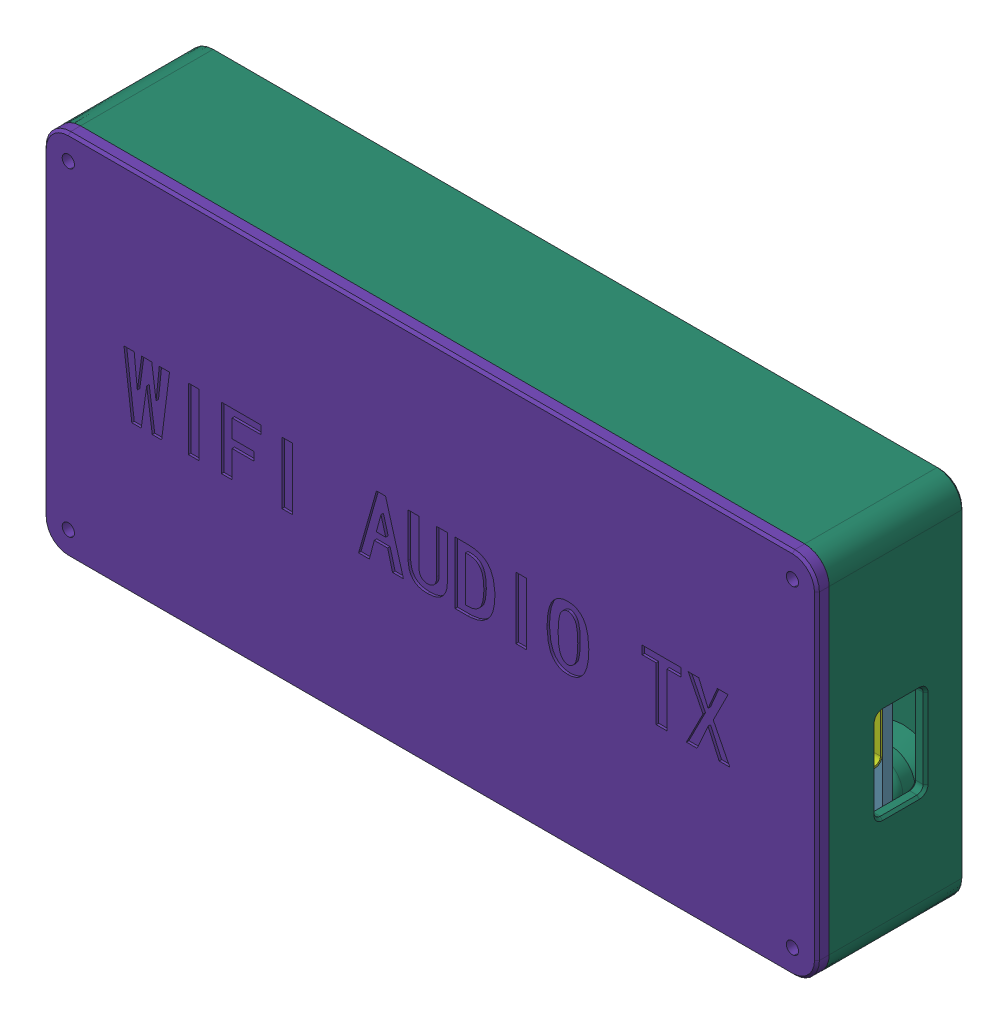
SolidWorks assembly WIFI-AUDIO-T, configuration 默认. Lengths in mm.
Overall size (126 64 24).
71 component instances, 17 part files, 8 mates.
Components (placement in the parent):
- 3D_WIFI-TX_2025-06-08.step-1: 3D_WIFI-TX_2025-06-08.step [默认] at (-69.7643 -55.4753 116.3565) size (116.36 41.38 15.8)
  - RN4~RES-ARRAY-SMD_0603-8P-L3.2-W1.6-BL~R0603-8P_L3.2-W1.6-H0.6~j3kg.step-1: RN4~RES-ARRAY-SMD_0603-8P-L3.2-W1.6-BL~R0603-8P_L3.2-W1.6-H0.6~j3kg.step [默认] at (69.0881 62.1031 1.6001) size (3.2 1.6 0.5)
    - RES-ARRAY-SMD_0603-8P-L3.2-W1.6-BL~R0603-8P_L3.2-W1.6-H0.6~j3kg.step-1: RES-ARRAY-SMD_0603-8P-L3.2-W1.6-BL~R0603-8P_L3.2-W1.6-H0.6~j3kg.step [默认] at origin size (3.2 1.6 0.5)
  - C50~C0603~C0603_L1.6-W0.8-H0.8~j3kg.step-1: C50~C0603~C0603_L1.6-W0.8-H0.8~j3kg.step [默认] at (86.1062 69.7231 1.6001) x (0 -1 0) z (0 0 1) size (1.6 0.8 0.8)
    - C0603~C0603_L1.6-W0.8-H0.8~j3kg.step-1: C0603~C0603_L1.6-W0.8-H0.8~j3kg.step [默认] at origin size (1.6 0.8 0.8)
  - C50~C0603~C0603_L1.6-W0.8-H0.8~j3kg.step-2: C50~C0603~C0603_L1.6-W0.8-H0.8~j3kg.step [默认] at (62.1031 47.1171 1.6001) x (0 1 0) z (0 0 1) size (1.6 0.8 0.8)
    - C0603~C0603_L1.6-W0.8-H0.8~j3kg.step-1: C0603~C0603_L1.6-W0.8-H0.8~j3kg.step [默认] at origin size (1.6 0.8 0.8)
  - C50~C0603~C0603_L1.6-W0.8-H0.8~j3kg.step-3: C50~C0603~C0603_L1.6-W0.8-H0.8~j3kg.step [默认] at (57.4041 63.6271 1.6001) x (0 -1 0) z (0 0 1) size (1.6 0.8 0.8)
    - C0603~C0603_L1.6-W0.8-H0.8~j3kg.step-1: C0603~C0603_L1.6-W0.8-H0.8~j3kg.step [默认] at origin size (1.6 0.8 0.8)
  - C50~C0603~C0603_L1.6-W0.8-H0.8~j3kg.step-4: C50~C0603~C0603_L1.6-W0.8-H0.8~j3kg.step [默认] at (53.5941 47.1171 1.6001) x (0 -1 0) z (0 0 1) size (1.6 0.8 0.8)
    - C0603~C0603_L1.6-W0.8-H0.8~j3kg.step-1: C0603~C0603_L1.6-W0.8-H0.8~j3kg.step [默认] at origin size (1.6 0.8 0.8)
  - C50~C0603~C0603_L1.6-W0.8-H0.8~j3kg.step-5: C50~C0603~C0603_L1.6-W0.8-H0.8~j3kg.step [默认] at (53.4671 63.6271 1.6001) x (0 1 0) z (0 0 1) size (1.6 0.8 0.8)
    - C0603~C0603_L1.6-W0.8-H0.8~j3kg.step-1: C0603~C0603_L1.6-W0.8-H0.8~j3kg.step [默认] at origin size (1.6 0.8 0.8)
  - C50~C0603~C0603_L1.6-W0.8-H0.8~j3kg.step-6: C50~C0603~C0603_L1.6-W0.8-H0.8~j3kg.step [默认] at (55.6261 47.2441 1.6001) x (0 -1 0) z (0 0 1) size (1.6 0.8 0.8)
    - C0603~C0603_L1.6-W0.8-H0.8~j3kg.step-1: C0603~C0603_L1.6-W0.8-H0.8~j3kg.step [默认] at origin size (1.6 0.8 0.8)
  - C50~C0603~C0603_L1.6-W0.8-H0.8~j3kg.step-7: C50~C0603~C0603_L1.6-W0.8-H0.8~j3kg.step [默认] at (55.3721 63.6271 1.6001) x (0 1 0) z (0 0 1) size (1.6 0.8 0.8)
    - C0603~C0603_L1.6-W0.8-H0.8~j3kg.step-1: C0603~C0603_L1.6-W0.8-H0.8~j3kg.step [默认] at origin size (1.6 0.8 0.8)
  - C50~C0603~C0603_L1.6-W0.8-H0.8~j3kg.step-8: C50~C0603~C0603_L1.6-W0.8-H0.8~j3kg.step [默认] at (46.2281 62.9921 1.6001) x (0 1 0) z (0 0 1) size (1.6 0.8 0.8)
    - C0603~C0603_L1.6-W0.8-H0.8~j3kg.step-1: C0603~C0603_L1.6-W0.8-H0.8~j3kg.step [默认] at origin size (1.6 0.8 0.8)
  - C50~C0603~C0603_L1.6-W0.8-H0.8~j3kg.step-9: C50~C0603~C0603_L1.6-W0.8-H0.8~j3kg.step [默认] at (46.2281 46.9901 1.6001) x (0 1 0) z (0 0 1) size (1.6 0.8 0.8)
    - C0603~C0603_L1.6-W0.8-H0.8~j3kg.step-1: C0603~C0603_L1.6-W0.8-H0.8~j3kg.step [默认] at origin size (1.6 0.8 0.8)
  - C50~C0603~C0603_L1.6-W0.8-H0.8~j3kg.step-10: C50~C0603~C0603_L1.6-W0.8-H0.8~j3kg.step [默认] at (88.2652 73.2791 1.6001) x (0 -1 0) z (0 0 1) size (1.6 0.8 0.8)
    - C0603~C0603_L1.6-W0.8-H0.8~j3kg.step-1: C0603~C0603_L1.6-W0.8-H0.8~j3kg.step [默认] at origin size (1.6 0.8 0.8)
  - C51~CAP-SMD_BD6.3-L6.6-W6.6-FD~CAP-SMD_BD6.3-L6.6-W6.6-FD~j3kg.step-1: C51~CAP-SMD_BD6.3-L6.6-W6.6-FD~CAP-SMD_BD6.3-L6.6-W6.6-FD~j3kg.step [默认] at (95.3772 48.2601 1.6001) size (7.8 6.6 7.75)
    - CAP-SMD_BD6.3-L6.6-W6.6-FD~CAP-SMD_BD6.3-L6.6-W6.6-FD~j3kg.step-1: CAP-SMD_BD6.3-L6.6-W6.6-FD~CAP-SMD_BD6.3-L6.6-W6.6-FD~j3kg.step [默认] at origin size (7.8 6.6 7.75)
  - C51~CAP-SMD_BD6.3-L6.6-W6.6-FD~CAP-SMD_BD6.3-L6.6-W6.6-FD~j3kg.step-2: C51~CAP-SMD_BD6.3-L6.6-W6.6-FD~CAP-SMD_BD6.3-L6.6-W6.6-FD~j3kg.step [默认] at (95.3772 40.7671 1.6001) size (7.8 6.6 7.75)
    - CAP-SMD_BD6.3-L6.6-W6.6-FD~CAP-SMD_BD6.3-L6.6-W6.6-FD~j3kg.step-1: CAP-SMD_BD6.3-L6.6-W6.6-FD~CAP-SMD_BD6.3-L6.6-W6.6-FD~j3kg.step [默认] at origin size (7.8 6.6 7.75)
  - C51~CAP-SMD_BD6.3-L6.6-W6.6-FD~CAP-SMD_BD6.3-L6.6-W6.6-FD~j3kg.step-3: C51~CAP-SMD_BD6.3-L6.6-W6.6-FD~CAP-SMD_BD6.3-L6.6-W6.6-FD~j3kg.step [默认] at (50.2921 40.6401 1.6001) size (7.8 6.6 7.75)
    - CAP-SMD_BD6.3-L6.6-W6.6-FD~CAP-SMD_BD6.3-L6.6-W6.6-FD~j3kg.step-1: CAP-SMD_BD6.3-L6.6-W6.6-FD~CAP-SMD_BD6.3-L6.6-W6.6-FD~j3kg.step [默认] at origin size (7.8 6.6 7.75)
  - C51~CAP-SMD_BD6.3-L6.6-W6.6-FD~CAP-SMD_BD6.3-L6.6-W6.6-FD~j3kg.step-4: C51~CAP-SMD_BD6.3-L6.6-W6.6-FD~CAP-SMD_BD6.3-L6.6-W6.6-FD~j3kg.step [默认] at (50.1651 69.9771 1.6001) size (7.8 6.6 7.75)
    - CAP-SMD_BD6.3-L6.6-W6.6-FD~CAP-SMD_BD6.3-L6.6-W6.6-FD~j3kg.step-1: CAP-SMD_BD6.3-L6.6-W6.6-FD~CAP-SMD_BD6.3-L6.6-W6.6-FD~j3kg.step [默认] at origin size (7.8 6.6 7.75)
  - C51~CAP-SMD_BD6.3-L6.6-W6.6-FD~CAP-SMD_BD6.3-L6.6-W6.6-FD~j3kg.step-5: C51~CAP-SMD_BD6.3-L6.6-W6.6-FD~CAP-SMD_BD6.3-L6.6-W6.6-FD~j3kg.step [默认] at (61.7221 40.3861 1.6001) x (-1 0 0) z (0 0 1) size (7.8 6.6 7.75)
    - CAP-SMD_BD6.3-L6.6-W6.6-FD~CAP-SMD_BD6.3-L6.6-W6.6-FD~j3kg.step-1: CAP-SMD_BD6.3-L6.6-W6.6-FD~CAP-SMD_BD6.3-L6.6-W6.6-FD~j3kg.step [默认] at origin size (7.8 6.6 7.75)
  - C51~CAP-SMD_BD6.3-L6.6-W6.6-FD~CAP-SMD_BD6.3-L6.6-W6.6-FD~j3kg.step-6: C51~CAP-SMD_BD6.3-L6.6-W6.6-FD~CAP-SMD_BD6.3-L6.6-W6.6-FD~j3kg.step [默认] at (60.0711 69.9771 1.6001) size (7.8 6.6 7.75)
    - CAP-SMD_BD6.3-L6.6-W6.6-FD~CAP-SMD_BD6.3-L6.6-W6.6-FD~j3kg.step-1: CAP-SMD_BD6.3-L6.6-W6.6-FD~CAP-SMD_BD6.3-L6.6-W6.6-FD~j3kg.step [默认] at origin size (7.8 6.6 7.75)
  - C51~CAP-SMD_BD6.3-L6.6-W6.6-FD~CAP-SMD_BD6.3-L6.6-W6.6-FD~j3kg.step-7: C51~CAP-SMD_BD6.3-L6.6-W6.6-FD~CAP-SMD_BD6.3-L6.6-W6.6-FD~j3kg.step [默认] at (79.1212 70.3581 1.6001) x (0 -1 0) z (0 0 1) size (7.8 6.6 7.75)
    - CAP-SMD_BD6.3-L6.6-W6.6-FD~CAP-SMD_BD6.3-L6.6-W6.6-FD~j3kg.step-1: CAP-SMD_BD6.3-L6.6-W6.6-FD~CAP-SMD_BD6.3-L6.6-W6.6-FD~j3kg.step [默认] at origin size (7.8 6.6 7.75)
  - R32~R0603~R0603~j3kg.step-1: R32~R0603~R0603~j3kg.step [默认] at (88.2652 69.7231 1.6001) x (0 1 0) z (0 0 1) size (1.62 0.81 0.45)
    - R0603~R0603~j3kg.step-1: R0603~R0603~j3kg.step [默认] at origin size (1.62 0.81 0.45)
  - R32~R0603~R0603~j3kg.step-2: R32~R0603~R0603~j3kg.step [默认] at (87.5032 63.3731 1.6001) x (-1 0 0) z (0 0 1) size (1.62 0.81 0.45)
    - R0603~R0603~j3kg.step-1: R0603~R0603~j3kg.step [默认] at origin size (1.62 0.81 0.45)
  - R34~RES-ADJ-TH_3P-L10.0-W10.0-P2.50-BL-BS~3296W~j3kg.step-1: R34~RES-ADJ-TH_3P-L10.0-W10.0-P2.50-BL-BS~3296W~j3kg.step [默认] at (20.955 63.1191 1.6001) x (-1 0 0) z (0 0 1) size (4.85 9.5 15)
    - RES-ADJ-TH_3P-L10.0-W10.0-P2.50-BL-BS~3296W~j3kg.step-1: RES-ADJ-TH_3P-L10.0-W10.0-P2.50-BL-BS~3296W~j3kg.step [默认] at origin size (4.85 9.5 15)
  - R34~RES-ADJ-TH_3P-L10.0-W10.0-P2.50-BL-BS~3296W~j3kg.step-2: R34~RES-ADJ-TH_3P-L10.0-W10.0-P2.50-BL-BS~3296W~j3kg.step [默认] at (20.701 47.1171 1.6001) x (-1 0 0) z (0 0 1) size (4.85 9.5 15)
    - RES-ADJ-TH_3P-L10.0-W10.0-P2.50-BL-BS~3296W~j3kg.step-1: RES-ADJ-TH_3P-L10.0-W10.0-P2.50-BL-BS~3296W~j3kg.step [默认] at origin size (4.85 9.5 15)
  - SETTING0~CONN-TH_2P-P2.50_HX25003-2A~CONN-TH_2P-P2.50_HX25003-2A~j3kg.step-1: SETTING0~CONN-TH_2P-P2.50_HX25003-2A~CONN-TH_2P-P2.50_HX25003-2A~j3kg.step [默认] at (78.9942 60.4521 1.6001) size (7.5 5.9 10.6)
    - CONN-TH_2P-P2.50_HX25003-2A~CONN-TH_2P-P2.50_HX25003-2A~j3kg.step-1: CONN-TH_2P-P2.50_HX25003-2A~CONN-TH_2P-P2.50_HX25003-2A~j3kg.step [默认] at origin size (7.5 5.9 10.6)
  - USB1~USB-C-SMD_TYPE-C-6PIN-2MD-073~USB-C-SMD_TYPE-C-6PIN-2MD-073~j3kg.step-1: USB1~USB-C-SMD_TYPE-C-6PIN-2MD-073~USB-C-SMD_TYPE-C-6PIN-2MD-073~j3kg.step [默认] at (118.1102 47.1171 1.6001) x (0 1 0) z (0 0 1) size (8.95 7.58 4.16)
    - USB-C-SMD_TYPE-C-6PIN-2MD-073~USB-C-SMD_TYPE-C-6PIN-2MD-073~j3kg.step-1: USB-C-SMD_TYPE-C-6PIN-2MD-073~USB-C-SMD_TYPE-C-6PIN-2MD-073~j3kg.step [默认] at origin size (8.95 7.58 4.16)
  - U14~CONN-TH_5P-P2.50_ZX-XH2.54-5PZZ~CONN-TH_5P-P2.50_ZX-XH2.54-5PZZ~j3kg.step-1: U14~CONN-TH_5P-P2.50_ZX-XH2.54-5PZZ~CONN-TH_5P-P2.50_ZX-XH2.54-5PZZ~j3kg.step [默认] at (118.6182 61.8491 1.6001) x (0 -1 0) z (0 0 1) size (15 5.91 10.4)
    - CONN-TH_5P-P2.50_ZX-XH2.54-5PZZ~CONN-TH_5P-P2.50_ZX-XH2.54-5PZZ~j3kg.step-1: CONN-TH_5P-P2.50_ZX-XH2.54-5PZZ~CONN-TH_5P-P2.50_ZX-XH2.54-5PZZ~j3kg.step [默认] at origin size (15 5.91 10.4)
  - U18~XFMR-SMD_L10.5-W8.0-P5.00-LS14.0_ED8-600~XFMR-SMD_L10.5-W8.0-P5.00-LS14.0_ED8-600~j3kg.step-1: U18~XFMR-SMD_L10.5-W8.0-P5.00-LS14.0_ED8-600~XFMR-SMD_L10.5-W8.0-P5.00-LS14.0_ED8-600~j3kg.step [默认] at (34.4171 62.9921 1.6001) x (0 -1 0) z (0 0 1) size (8.01 14 5.02)
    - XFMR-SMD_L10.5-W8.0-P5.00-LS14.0_ED8-600~XFMR-SMD_L10.5-W8.0-P5.00-LS14.0_ED8-600~j3kg.step-1: XFMR-SMD_L10.5-W8.0-P5.00-LS14.0_ED8-600~XFMR-SMD_L10.5-W8.0-P5.00-LS14.0_ED8-600~j3kg.step [默认] at origin size (8.01 14 5.02)
  - U18~XFMR-SMD_L10.5-W8.0-P5.00-LS14.0_ED8-600~XFMR-SMD_L10.5-W8.0-P5.00-LS14.0_ED8-600~j3kg.step-2: U18~XFMR-SMD_L10.5-W8.0-P5.00-LS14.0_ED8-600~XFMR-SMD_L10.5-W8.0-P5.00-LS14.0_ED8-600~j3kg.step [默认] at (34.4171 47.1171 1.6001) x (0 -1 0) z (0 0 1) size (8.01 14 5.02)
    - XFMR-SMD_L10.5-W8.0-P5.00-LS14.0_ED8-600~XFMR-SMD_L10.5-W8.0-P5.00-LS14.0_ED8-600~j3kg.step-1: XFMR-SMD_L10.5-W8.0-P5.00-LS14.0_ED8-600~XFMR-SMD_L10.5-W8.0-P5.00-LS14.0_ED8-600~j3kg.step [默认] at origin size (8.01 14 5.02)
  - U21~WIFI-SMD_ESP32-WROOM-32UE~WIFI-SMD_L19.2-18.0-H3.2-ESP32-WROOM-32UE~j3kg.step-1: U21~WIFI-SMD_ESP32-WROOM-32UE~WIFI-SMD_L19.2-18.0-H3.2-ESP32-WROOM-32UE~j3kg.step [默认] at (101.4732 64.7701 1.6001) size (18 19.2 3.2)
    - WIFI-SMD_ESP32-WROOM-32UE~WIFI-SMD_L19.2-18.0-H3.2-ESP32-WROOM-32UE~j3kg.step-1: WIFI-SMD_ESP32-WROOM-32UE~WIFI-SMD_L19.2-18.0-H3.2-ESP32-WROOM-32UE~j3kg.step [默认] at origin size (18 19.2 3.2)
  - U9~CONN-TH_P5.00_KF301-5.0-2P~CONN-TH_P5.00_KF301-5.0-2P~j3kg.step-1: U9~CONN-TH_P5.00_KF301-5.0-2P~CONN-TH_P5.00_KF301-5.0-2P~j3kg.step [默认] at (10.541 47.1171 1.6001) x (0 -1 0) z (0 0 1) size (10.4 7.46 13.15)
    - CONN-TH_P5.00_KF301-5.0-2P~CONN-TH_P5.00_KF301-5.0-2P~j3kg.step-1: CONN-TH_P5.00_KF301-5.0-2P~CONN-TH_P5.00_KF301-5.0-2P~j3kg.step [默认] at origin size (10.4 7.46 13.15)
  - U9~CONN-TH_P5.00_KF301-5.0-2P~CONN-TH_P5.00_KF301-5.0-2P~j3kg.step-2: U9~CONN-TH_P5.00_KF301-5.0-2P~CONN-TH_P5.00_KF301-5.0-2P~j3kg.step [默认] at (10.541 63.1191 1.6001) x (0 -1 0) z (0 0 1) size (10.4 7.46 13.15)
    - CONN-TH_P5.00_KF301-5.0-2P~CONN-TH_P5.00_KF301-5.0-2P~j3kg.step-1: CONN-TH_P5.00_KF301-5.0-2P~CONN-TH_P5.00_KF301-5.0-2P~j3kg.step [默认] at origin size (10.4 7.46 13.15)
  - U9~CONN-TH_P5.00_KF301-5.0-2P~CONN-TH_P5.00_KF301-5.0-2P~j3kg.step-3: U9~CONN-TH_P5.00_KF301-5.0-2P~CONN-TH_P5.00_KF301-5.0-2P~j3kg.step [默认] at (106.6802 40.8941 1.6001) size (10.4 7.46 13.15)
    - CONN-TH_P5.00_KF301-5.0-2P~CONN-TH_P5.00_KF301-5.0-2P~j3kg.step-1: CONN-TH_P5.00_KF301-5.0-2P~CONN-TH_P5.00_KF301-5.0-2P~j3kg.step [默认] at origin size (10.4 7.46 13.15)
  - U16~SSOP-28_L10.2-W5.3-P0.65-LS7.8-BL~SSOP-28_L10.2-W5.3-H2.0-LS7.8-P0.65~j3kg.step-1: U16~SSOP-28_L10.2-W5.3-P0.65-LS7.8-BL~SSOP-28_L10.2-W5.3-H2.0-LS7.8-P0.65~j3kg.step [默认] at (58.0391 55.4991 1.6001) size (10.2 7.8 2.2)
    - SSOP-28_L10.2-W5.3-P0.65-LS7.8-BL~SSOP-28_L10.2-W5.3-H2.0-LS7.8-P0.65~j3kg.step-1: SSOP-28_L10.2-W5.3-P0.65-LS7.8-BL~SSOP-28_L10.2-W5.3-H2.0-LS7.8-P0.65~j3kg.step [默认] at origin size (10.2 7.8 2.2)
  - U20~TO-263-3_L8.6-W10.2-P2.54-LS14.4-BR~TO-263-3_L10.2-W8.7-H4.5-LS14.4-P2.54~j3kg.step-1: U20~TO-263-3_L8.6-W10.2-P2.54-LS14.4-BR~TO-263-3_L10.2-W8.7-H4.5-LS14.4-P2.54~j3kg.step [默认] at (81.9822 44.4738 1.6001) size (14.23 10.2 4.5)
    - TO-263-3_L8.6-W10.2-P2.54-LS14.4-BR~TO-263-3_L10.2-W8.7-H4.5-LS14.4-P2.54~j3kg.step-1: TO-263-3_L8.6-W10.2-P2.54-LS14.4-BR~TO-263-3_L10.2-W8.7-H4.5-LS14.4-P2.54~j3kg.step [默认] at origin size (14.23 10.2 4.5)
  - Board~j3kg.step-1: Board~j3kg.step [默认] at origin size (116.31 41.38 1.6)
- WIFI-AUDIO-T-BOX-1: WIFI-AUDIO-T-BOX [默认] at (-68.0206 -34.7959 109.3565) x (1 0 0) z (0 -1 0) size (126 22 60)
- sma座-1: sma座 [默认] at (42.9794 -32.7959 122.3565) x (-0.837169 0 -0.546944) z (-0.546944 0 0.837169) size (10 36 10)
- WIFI-AUDIO-T-BOX1-1: WIFI-AUDIO-T-BOX1 [默认] at (-68.0206 -34.7959 131.3565) x (1 0 0) z (0 -1 0) size (126 2 60)
Mates (geometry in assembly coordinates):
- 距离2: distance = 5 mm anti-aligned: plane of WIFI-AUDIO-T-BOX-1 through (-68.0206 -34.7959 111.3565) normal (0 0 1); plane of 3D_WIFI-TX_2025-06-08.step-1/Board~j3kg.step-1 through (-4.8672 -0.4842 116.3565) normal (0 0 -1)
- 距离3: distance = 5 mm aligned: plane of 3D_WIFI-TX_2025-06-08.step-1/Board~j3kg.step-1 through (-63.0206 20.2041 116.3565) normal (0 1 0); plane of WIFI-AUDIO-T-BOX-1 through (-68.0206 25.2041 111.3565) normal (0 1 0)
- 距离4: distance = 5 mm aligned: plane of 3D_WIFI-TX_2025-06-08.step-1/Board~j3kg.step-1 through (-63.0206 -21.1726 116.3565) normal (-1 0 0); plane of WIFI-AUDIO-T-BOX-1 through (-68.0206 -34.7959 111.3565) normal (-1 0 0)
- 同心1: concentric aligned: cylinder of WIFI-AUDIO-T-BOX-1 through (42.9794 -32.7959 122.3565) axis (0 -1 0) radius 3.25; cylinder of sma座-1 through (42.9794 -2.7959 122.3565) axis (0 -1 0) radius 1
- 重合7: coincident anti-aligned: plane of WIFI-AUDIO-T-BOX-1 through (-66.0206 -32.7959 131.3565) normal (0 1 0); plane of sma座-1 through (42.9794 -32.7959 122.3565) normal (0 -1 0)
- 重合8: coincident anti-aligned: plane of WIFI-AUDIO-T-BOX-1 through (-68.0206 -34.7959 131.3565) normal (0 0 1); plane of WIFI-AUDIO-T-BOX1-1 through (53.9794 21.2041 131.3565) normal (0 0 -1)
- 重合9: coincident aligned: plane of WIFI-AUDIO-T-BOX-1 through (-68.0206 -34.7959 111.3565) normal (-1 0 0); plane of WIFI-AUDIO-T-BOX1-1 through (-68.0206 -30.7959 133.3565) normal (-1 0 0)
- 重合10: coincident aligned: plane of WIFI-AUDIO-T-BOX-1 through (-68.0206 -34.7959 111.3565) normal (0 -1 0); plane of WIFI-AUDIO-T-BOX1-1 through (-64.0206 -34.7959 133.3565) normal (0 -1 0)
